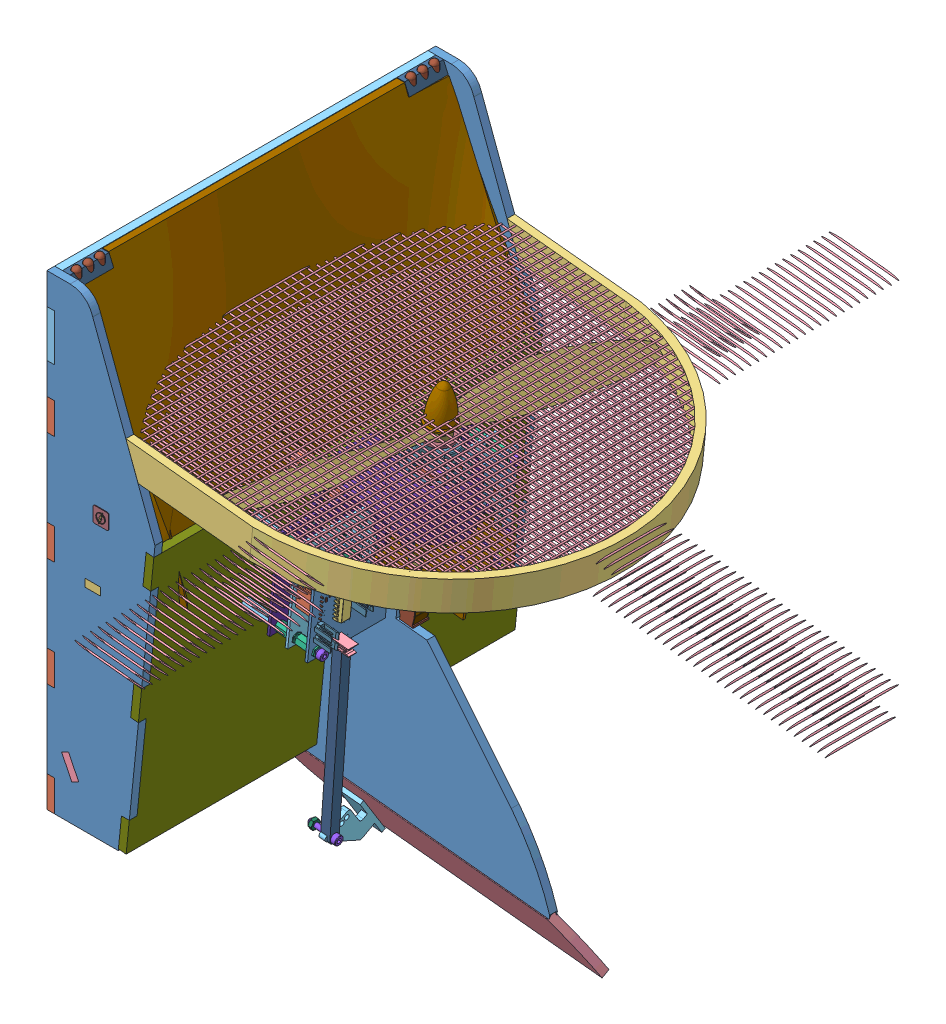
SolidWorks assembly AssTotaleSimu8, configuration Défaut. Lengths in mm. (continued)
Components (placement in the parent): (continued)
- AssStructSimu-1: AssStructSimu [Défaut] at (-125.7658 -1.8483 624.6548) x (1 0 0) z (0 0 -1) size (253.25 324.59 251.6) (continued)
  - AssCarte-1: AssCarte [Défaut] at (-42.8534 32.2132 302.028) x (-0.101852 0.9948 0) z (0.9948 0.101852 0) size (67.15 130.57 98.45) (continued)
    - carte_onduleur_v4-1: carte_onduleur_v4 [Défaut] at (-25.7639 0.8332 112.9379) size (66.52 130.57 82.34) (continued)
      - CARTE_ALIM-1: CARTE_ALIM [Défaut] at (-6.4 -57.2 0.803) size (60 130 18.35) (continued)
        - Open CASCADE STEP translator 6.8 1.63.1-1: Open CASCADE STEP translator 6.8 1.63.1 [Défaut] at origin size (60 130 18.35) (continued)
          - Body_1_6-1: Body_1_6 [Défaut] at (7 56 -12) size (60 130 18.35) (continued)
            - 109-1: 109 [Défaut] at (25.4933 -41.1272 0.803) x (-1 0 0) z (0 0 1) size (2.34 1.04 0.5) (continued)
              - =_[0_1_1_45]-1: =_[0_1_1_45] [Défaut] at origin size (2.34 1.04 0.5) (continued)
                - 49_3-1: 49_3 [Défaut] at origin size (2.29 1.04 0.43)
                - 50-1: 50 [Défaut] at (0.3048 0 0) x (-1 0 0) z (0 0 1) size (0.51 1.02 0.5)
                - 51-1: 51 [Défaut] at origin size (0.51 1.02 0.5)
            - 111-1: 111 [Défaut] at (22.0269 -41.8272 0.803) x (-1 0 0) z (0 0 1) size (2.34 1.04 0.5)
              - =_[0_1_1_45]-1: =_[0_1_1_45] [Défaut] at origin size (2.34 1.04 0.5)
                - 49_3-1: 49_3 [Défaut] at origin size (2.29 1.04 0.43)
                - 50-1: 50 [Défaut] at (0.3048 0 0) x (-1 0 0) z (0 0 1) size (0.51 1.02 0.5)
                - 51-1: 51 [Défaut] at origin size (0.51 1.02 0.5)
            - 113-1: 113 [Défaut] at (-24.8 -36.7036 0.803) x (0 1 0) z (0 0 1) size (2.34 1.04 0.5)
              - =_[0_1_1_45]-1: =_[0_1_1_45] [Défaut] at origin size (2.34 1.04 0.5)
                - 49_3-1: 49_3 [Défaut] at origin size (2.29 1.04 0.43)
                - 50-1: 50 [Défaut] at (0.3048 0 0) x (-1 0 0) z (0 0 1) size (0.51 1.02 0.5)
                - 51-1: 51 [Défaut] at origin size (0.51 1.02 0.5)
            - 115-1: 115 [Défaut] at (-24.8 -40.3036 0.803) x (0 1 0) z (0 0 1) size (2.34 1.04 0.5)
              - =_[0_1_1_45]-1: =_[0_1_1_45] [Défaut] at origin size (2.34 1.04 0.5)
                - 49_3-1: 49_3 [Défaut] at origin size (2.29 1.04 0.43)
                - 50-1: 50 [Défaut] at (0.3048 0 0) x (-1 0 0) z (0 0 1) size (0.51 1.02 0.5)
                - 51-1: 51 [Défaut] at origin size (0.51 1.02 0.5)
            - 117-1: 117 [Défaut] at (-16 -48.27 0.803) x (0 -1 0) z (0 0 1) size (2.34 1.04 0.5)
              - =_[0_1_1_45]-1: =_[0_1_1_45] [Défaut] at origin size (2.34 1.04 0.5)
                - 49_3-1: 49_3 [Défaut] at origin size (2.29 1.04 0.43)
                - 50-1: 50 [Défaut] at (0.3048 0 0) x (-1 0 0) z (0 0 1) size (0.51 1.02 0.5)
                - 51-1: 51 [Défaut] at origin size (0.51 1.02 0.5)
            - 119-1: 119 [Défaut] at (-22.5189 -47.87 0.803) x (-1 0 0) z (0 0 1) size (2.34 1.04 0.5)
              - =_[0_1_1_45]-1: =_[0_1_1_45] [Défaut] at origin size (2.34 1.04 0.5)
                - 49_3-1: 49_3 [Défaut] at origin size (2.29 1.04 0.43)
                - 50-1: 50 [Défaut] at (0.3048 0 0) x (-1 0 0) z (0 0 1) size (0.51 1.02 0.5)
                - 51-1: 51 [Défaut] at origin size (0.51 1.02 0.5)
            - 121-1: 121 [Défaut] at (22.3933 -38.9272 0.803) size (2.34 1.04 0.5)
              - =_[0_1_1_45]-1: =_[0_1_1_45] [Défaut] at origin size (2.34 1.04 0.5)
                - 49_3-1: 49_3 [Défaut] at origin size (2.29 1.04 0.43)
                - 50-1: 50 [Défaut] at (0.3048 0 0) x (-1 0 0) z (0 0 1) size (0.51 1.02 0.5)
                - 51-1: 51 [Défaut] at origin size (0.51 1.02 0.5)
            - 123-1: 123 [Défaut] at (22.0933 -36.4272 0.803) x (-1 0 0) z (0 0 1) size (2.34 1.04 0.5)
              - =_[0_1_1_45]-1: =_[0_1_1_45] [Défaut] at origin size (2.34 1.04 0.5)
                - 49_3-1: 49_3 [Défaut] at origin size (2.29 1.04 0.43)
                - 50-1: 50 [Défaut] at (0.3048 0 0) x (-1 0 0) z (0 0 1) size (0.51 1.02 0.5)
                - 51-1: 51 [Défaut] at origin size (0.51 1.02 0.5)
            - 125-1: 125 [Défaut] at (22.3933 -32.0272 0.803) x (0 -1 0) z (0 0 1) size (2.34 1.04 0.5)
              - =_[0_1_1_45]-1: =_[0_1_1_45] [Défaut] at origin size (2.34 1.04 0.5)
                - 49_3-1: 49_3 [Défaut] at origin size (2.29 1.04 0.43)
                - 50-1: 50 [Défaut] at (0.3048 0 0) x (-1 0 0) z (0 0 1) size (0.51 1.02 0.5)
                - 51-1: 51 [Défaut] at origin size (0.51 1.02 0.5)
            - 127-1: 127 [Défaut] at (17.9597 -23.1272 0.803) size (2.34 1.04 0.5)
              - =_[0_1_1_16]-1: =_[0_1_1_16] [Défaut] at origin size (2.34 1.04 0.5)
                - 14_2-1: 14_2 [Défaut] at origin size (2.29 1.04 0.43)
                - 15_2-1: 15_2 [Défaut] at (0.3048 0 0) x (-1 0 0) z (0 0 1) size (0.51 1.02 0.5)
                - 16_2-1: 16_2 [Défaut] at origin size (0.51 1.02 0.5)
            - 129-1: 129 [Défaut] at (20.0269 -24.9272 0.803) x (-1 0 0) z (0 0 1) size (2.34 1.04 0.5)
              - =_[0_1_1_16]-1: =_[0_1_1_16] [Défaut] at origin size (2.34 1.04 0.5)
                - 14_2-1: 14_2 [Défaut] at origin size (2.29 1.04 0.43)
                - 15_2-1: 15_2 [Défaut] at (0.3048 0 0) x (-1 0 0) z (0 0 1) size (0.51 1.02 0.5)
                - 16_2-1: 16_2 [Défaut] at origin size (0.51 1.02 0.5)
            - 131-1: 131 [Défaut] at (16.9933 -37.5272 0.803) x (-1 0 0) z (0 0 1) size (2.34 1.04 0.5)
              - =_[0_1_1_45]-1: =_[0_1_1_45] [Défaut] at origin size (2.34 1.04 0.5)
                - 49_3-1: 49_3 [Défaut] at origin size (2.29 1.04 0.43)
                - 50-1: 50 [Défaut] at (0.3048 0 0) x (-1 0 0) z (0 0 1) size (0.51 1.02 0.5)
                - 51-1: 51 [Défaut] at origin size (0.51 1.02 0.5)
            - 136-1: 136 [Défaut] at (3.2957 -29.23 0.803) x (-1 0 0) z (0 0 1) size (4.78 2.79 2.03)
              - =_[0_1_1_110]_2-1: =_[0_1_1_110]_2 [Défaut] at origin size (4.78 2.79 2.03)
                - 132-1: 132 [Défaut] at origin size (4.32 2.79 1.78)
                - 133-1: 133 [Défaut] at (0.4572 0 0) x (-1 0 0) z (0 0 1) size (1.02 1.27 1.32)
                - 134-1: 134 [Défaut] at origin size (1.02 1.27 1.32)
            - 141-1: 141 [Défaut] at (0.2436 -33.3673 0.803) size (3.35 1.3 0.55)
              - =_[0_1_1_115]_2-1: =_[0_1_1_115]_2 [Défaut] at origin size (3.35 1.3 0.55)
                - 137-1: 137 [Défaut] at origin size (3.3 1.3 0.48)
                - 138-1: 138 [Défaut] at (0.5588 0 0) x (-1 0 0) z (0 0 1) size (0.76 1.27 0.55)
                - 139-1: 139 [Défaut] at origin size (0.76 1.27 0.55)
            - 143_2-1: 143_2 [Défaut] at (-0.3 -45.47 0.803) x (0 1 0) z (0 0 1) size (2.34 1.04 0.5)
              - =_[0_1_1_16]-1: =_[0_1_1_16] [Défaut] at origin size (2.34 1.04 0.5)
                - 14_2-1: 14_2 [Défaut] at origin size (2.29 1.04 0.43)
                - 15_2-1: 15_2 [Défaut] at (0.3048 0 0) x (-1 0 0) z (0 0 1) size (0.51 1.02 0.5)
                - 16_2-1: 16_2 [Défaut] at origin size (0.51 1.02 0.5)
            - 145-1: 145 [Défaut] at (6.6 31.13 0.803) x (0 1 0) z (0 0 1) size (3.35 1.3 0.55)
              - =_[0_1_1_25]_2-1: =_[0_1_1_25]_2 [Défaut] at origin size (3.35 1.3 0.55)
                - 24-1: 24 [Défaut] at origin size (3.3 1.3 0.48)
                - 25_2-1: 25_2 [Défaut] at (0.5588 0 0) x (-1 0 0) z (0 0 1) size (0.76 1.27 0.55)
                - 26_2-1: 26_2 [Défaut] at origin size (0.76 1.27 0.55)
            - 148-1: 148 [Défaut] at (-7.5 -56.57 0.803) size (15.24 2.54 7.37)
              - =_[0_1_1_122]_2-1: =_[0_1_1_122]_2 [Défaut] at origin size (15.24 2.54 7.37)
                - 146-1: 146 [Défaut] at (6.3 0 1) x (1 0 0) z (0 -1 0) size (15.24 7.37 2.54)
            - 150-1: 150 [Défaut] at (-26.3 -45.9 0.803) x (0 1 0) z (0 0 1) size (2.34 1.04 0.5)
              - =_[0_1_1_45]-1: =_[0_1_1_45] [Défaut] at origin size (2.34 1.04 0.5)
                - 49_3-1: 49_3 [Défaut] at origin size (2.29 1.04 0.43)
                - 50-1: 50 [Défaut] at (0.3048 0 0) x (-1 0 0) z (0 0 1) size (0.51 1.02 0.5)
                - 51-1: 51 [Défaut] at origin size (0.51 1.02 0.5)
    - AssEntretoise-1: AssEntretoise [Défaut] at (-50.7639 -62.5535 129.2811) x (0 0 -1) z (1 0 0) size (58.24 7.29 7.81)
      - socket head cap screw 4762_din-1: socket head cap screw 4762_din [EN ISO 4762 M3 x 5 - 5N] at (-2.4967 0.5867 0) size (8 5.5 5.5)
      - hexagonal_spacer_MF_M3_H20_HEX5.5_FTD6_MTL6-1: hexagonal_spacer_MF_M3_H20_HEX5.5_FTD6_MTL6 [Défaut] at (48.3433 0.5867 0) x (0 0 1) z (-1 0 0) size (6.36 5.51 26)
      - hex nut style 1 gradeab_din-1: hex nut style 1 gradeab_din [Hexagon Nut ISO 4032 - M3 - W - N] at (53.3433 0.5867 0) x (0 0.943962 0.330053) z (-1 0 0) size (5.5 6.35 2.4)
      - hexagonal_spacer_MF_M3_H12_HEX5.5_FTD6_MTL6-2: hexagonal_spacer_MF_M3_H12_HEX5.5_FTD6_MTL6 [Défaut] at (27.0633 0.5867 0) x (0 0.248308 0.968681) z (-1 0 0) size (6.36 5.51 18)
      - hexagonal_spacer_MF_M3_H12_HEX5.5_FTD6_MTL6-3: hexagonal_spacer_MF_M3_H12_HEX5.5_FTD6_MTL6 [Défaut] at (13.7833 0.5867 0) x (0 0 1) z (-1 0 0) size (6.36 5.51 18)
    - AssEntretoise-2: AssEntretoise [Défaut] at (0.4521 -62.0374 129.2811) x (0 0 -1) z (0.694658 0.71934 0) size (58.24 7.29 7.81)
      - socket head cap screw 4762_din-1: socket head cap screw 4762_din [EN ISO 4762 M3 x 5 - 5N] at (-2.4967 0.5867 0) size (8 5.5 5.5)
      - hexagonal_spacer_MF_M3_H20_HEX5.5_FTD6_MTL6-1: hexagonal_spacer_MF_M3_H20_HEX5.5_FTD6_MTL6 [Défaut] at (48.3433 0.5867 0) x (0 0 1) z (-1 0 0) size (6.36 5.51 26)
      - hex nut style 1 gradeab_din-1: hex nut style 1 gradeab_din [Hexagon Nut ISO 4032 - M3 - W - N] at (53.3433 0.5867 0) x (0 0.943962 0.330053) z (-1 0 0) size (5.5 6.35 2.4)
      - hexagonal_spacer_MF_M3_H12_HEX5.5_FTD6_MTL6-2: hexagonal_spacer_MF_M3_H12_HEX5.5_FTD6_MTL6 [Défaut] at (27.0633 0.5867 0) x (0 0.248308 0.968681) z (-1 0 0) size (6.36 5.51 18)
      - hexagonal_spacer_MF_M3_H12_HEX5.5_FTD6_MTL6-3: hexagonal_spacer_MF_M3_H12_HEX5.5_FTD6_MTL6 [Défaut] at (13.7833 0.5867 0) x (0 0 1) z (-1 0 0) size (6.36 5.51 18)
    - AssEntretoise-3: AssEntretoise [Défaut] at (-51.9799 58.1038 129.2811) x (0 0 -1) z (-0.694658 -0.71934 0) size (58.24 7.29 7.81)
      - socket head cap screw 4762_din-1: socket head cap screw 4762_din [EN ISO 4762 M3 x 5 - 5N] at (-2.4967 0.5867 0) size (8 5.5 5.5)
      - hexagonal_spacer_MF_M3_H20_HEX5.5_FTD6_MTL6-1: hexagonal_spacer_MF_M3_H20_HEX5.5_FTD6_MTL6 [Défaut] at (48.3433 0.5867 0) x (0 0 1) z (-1 0 0) size (6.36 5.51 26)
      - hex nut style 1 gradeab_din-1: hex nut style 1 gradeab_din [Hexagon Nut ISO 4032 - M3 - W - N] at (53.3433 0.5867 0) x (0 0.943962 0.330053) z (-1 0 0) size (5.5 6.35 2.4)
      - hexagonal_spacer_MF_M3_H12_HEX5.5_FTD6_MTL6-2: hexagonal_spacer_MF_M3_H12_HEX5.5_FTD6_MTL6 [Défaut] at (27.0633 0.5867 0) x (0 0.248308 0.968681) z (-1 0 0) size (6.36 5.51 18)
      - hexagonal_spacer_MF_M3_H12_HEX5.5_FTD6_MTL6-3: hexagonal_spacer_MF_M3_H12_HEX5.5_FTD6_MTL6 [Défaut] at (13.7833 0.5867 0) x (0 0 1) z (-1 0 0) size (6.36 5.51 18)
    - AssEntretoise-4: AssEntretoise [Défaut] at (0.2897 58.1744 129.2811) x (0 0 -1) z (-0.999848 0.017452 0) size (58.24 7.29 7.81)
      - socket head cap screw 4762_din-1: socket head cap screw 4762_din [EN ISO 4762 M3 x 5 - 5N] at (-2.4967 0.5867 0) size (8 5.5 5.5)
      - hexagonal_spacer_MF_M3_H20_HEX5.5_FTD6_MTL6-1: hexagonal_spacer_MF_M3_H20_HEX5.5_FTD6_MTL6 [Défaut] at (48.3433 0.5867 0) x (0 0 1) z (-1 0 0) size (6.36 5.51 26)
      - hex nut style 1 gradeab_din-1: hex nut style 1 gradeab_din [Hexagon Nut ISO 4032 - M3 - W - N] at (53.3433 0.5867 0) x (0 0.943962 0.330053) z (-1 0 0) size (5.5 6.35 2.4)
      - hexagonal_spacer_MF_M3_H12_HEX5.5_FTD6_MTL6-2: hexagonal_spacer_MF_M3_H12_HEX5.5_FTD6_MTL6 [Défaut] at (27.0633 0.5867 0) x (0 0.248308 0.968681) z (-1 0 0) size (6.36 5.51 18)
      - hexagonal_spacer_MF_M3_H12_HEX5.5_FTD6_MTL6-3: hexagonal_spacer_MF_M3_H12_HEX5.5_FTD6_MTL6 [Défaut] at (13.7833 0.5867 0) x (0 0 1) z (-1 0 0) size (6.36 5.51 18)
    - AssMpu-1: AssMpu [Défaut] at (-44.7921 29.4106 121.7839) size (8 8 22.28)
      - hex nut style 1 gradeab_din-1: hex nut style 1 gradeab_din [Hexagon Nut ISO 4032 - M3 - W - N] at (0.2783 0.3227 1.2) size (5.5 6.35 2.4)
      - plain washer 6903 type ab_din-1: plain washer 6903 type ab_din [DIN 6903-A3] at (0.2783 0.3227 1.2) x (0 0 1) z (-1 0 0) size (1 8 8)
      - socket head cap screw 4762_din-1: socket head cap screw 4762_din [EN ISO 4762 M3 x 5 - 5N] at (0.2783 0.3227 19.76) x (0 0 -1) z (-0.852155 0.523289 0) size (8 5.5 5.5)
      - hexagonal_spacer_MF_M3_H12_HEX5.5_FTD6_MTL6-1: hexagonal_spacer_MF_M3_H12_HEX5.5_FTD6_MTL6 [Défaut] at (0.2783 0.3227 3.48) size (6.36 5.51 18)
    - AssMpu-2: AssMpu [Défaut] at (-24.7921 29.4106 121.7839) size (8 8 22.28)
      - hex nut style 1 gradeab_din-1: hex nut style 1 gradeab_din [Hexagon Nut ISO 4032 - M3 - W - N] at (0.2783 0.3227 1.2) size (5.5 6.35 2.4)
      - plain washer 6903 type ab_din-1: plain washer 6903 type ab_din [DIN 6903-A3] at (0.2783 0.3227 1.2) x (0 0 1) z (-1 0 0) size (1 8 8)
      - socket head cap screw 4762_din-1: socket head cap screw 4762_din [EN ISO 4762 M3 x 5 - 5N] at (0.2783 0.3227 19.76) x (0 0 -1) z (-0.852155 0.523289 0) size (8 5.5 5.5)
      - hexagonal_spacer_MF_M3_H12_HEX5.5_FTD6_MTL6-1: hexagonal_spacer_MF_M3_H12_HEX5.5_FTD6_MTL6 [Défaut] at (0.2783 0.3227 3.48) size (6.36 5.51 18)
    - AssCosse-1: AssCosse [Défaut] at (-36.6204 16.2367 163.5671) x (0 1 0) z (-0.344896 0 0.938641) size (9.83 18.66 11.64)
      - socket head cap screw 4762_din-1: socket head cap screw 4762_din [EN ISO 4762 M3 x 6 - 6N] at (-5.1064 0.3659 0) size (9 5.5 5.5)
      - plain washer 6903 type ab_din-1: plain washer 6903 type ab_din [DIN 6903-A3] at (-2.1064 0.3659 0) size (1 8 8)
      - hex nut style 1 gradeab_din-2: hex nut style 1 gradeab_din [Hexagon Nut ISO 4032 - M3 - W - N] at (1.281 0.3659 0) x (0 0.924225 0.381849) z (-1 0 0) size (5.5 6.35 2.4)
      - 31880-1: 31880 [Default] at (0.4936 0.3659 0) x (0 0.344896 -0.938641) z (0 -0.938641 -0.344896) size (5.54 5 17.37)
    - AssCosse-2: AssCosse [Défaut] at (-36.6204 1.2367 163.5671) x (0 1 0) z (-0.344896 0 0.938641) size (9.83 18.66 11.64)
      - socket head cap screw 4762_din-1: socket head cap screw 4762_din [EN ISO 4762 M3 x 6 - 6N] at (-5.1064 0.3659 0) size (9 5.5 5.5)
      - plain washer 6903 type ab_din-1: plain washer 6903 type ab_din [DIN 6903-A3] at (-2.1064 0.3659 0) size (1 8 8)
      - hex nut style 1 gradeab_din-2: hex nut style 1 gradeab_din [Hexagon Nut ISO 4032 - M3 - W - N] at (1.281 0.3659 0) x (0 0.924225 0.381849) z (-1 0 0) size (5.5 6.35 2.4)
      - 31880-1: 31880 [Default] at (0.4936 0.3659 0) x (0 0.344896 -0.938641) z (0 -0.938641 -0.344896) size (5.54 5 17.37)
    - AssCosse-3: AssCosse [Défaut] at (-36.6204 -13.7633 163.5671) x (0 1 0) z (-0.344896 0 0.938641) size (9.83 18.66 11.64)
      - socket head cap screw 4762_din-1: socket head cap screw 4762_din [EN ISO 4762 M3 x 6 - 6N] at (-5.1064 0.3659 0) size (9 5.5 5.5)
      - plain washer 6903 type ab_din-1: plain washer 6903 type ab_din [DIN 6903-A3] at (-2.1064 0.3659 0) size (1 8 8)
      - hex nut style 1 gradeab_din-2: hex nut style 1 gradeab_din [Hexagon Nut ISO 4032 - M3 - W - N] at (1.281 0.3659 0) x (0 0.924225 0.381849) z (-1 0 0) size (5.5 6.35 2.4)
      - 31880-1: 31880 [Default] at (0.4936 0.3659 0) x (0 0.344896 -0.938641) z (0 -0.938641 -0.344896) size (5.54 5 17.37)
    - Terminal_QD_Female-1: Terminal_QD_Female [Default] at (-33.4139 20.2862 128.1409) x (0 1 0) z (-1 0 0) size (9.4 5.5 22.35)
    - Terminal_QD_Female-2: Terminal_QD_Female [Default] at (-33.4139 5.2862 128.1409) x (0 1 0) z (-1 0 0) size (9.4 5.5 22.35)
    - Terminal_QD_Female-3: Terminal_QD_Female [Default] at (-33.4139 -9.7138 128.1409) x (0 1 0) z (-1 0 0) size (9.4 5.5 22.35)
    - Terminal_QD_Female-4: Terminal_QD_Female [Default] at (-33.4139 -9.7138 145.1409) x (0 1 0) z (-1 0 0) size (9.4 5.5 22.35)
    - Terminal_QD_Female-5: Terminal_QD_Female [Default] at (-33.4139 5.2862 145.1409) x (0 1 0) z (-1 0 0) size (9.4 5.5 22.35)
    - Terminal_QD_Female-6: Terminal_QD_Female [Default] at (-33.4139 20.2862 145.1409) x (0 1 0) z (-1 0 0) size (9.4 5.5 22.35)
- AssTige-1: AssTige [Défaut] at (-241.576 -121.7726 340.4233) x (-0.101791 -0.994204 -0.034587) z (0.9948 -0.101852 0) size (166.39 7.19 19)
  - tige_servo-1: tige_servo [Défaut] at (-106.2712 0.2685 162) size (165 6 6)
  - socket head cap screw 4762_din-2: socket head cap screw 4762_din [EN ISO 4762 M2 x 10 - 10N] at (-104.2712 3.2685 170) x (0 0 -1) z (0.923728 0.383049 0) size (12 3.8 3.8)
  - hex nut style 1 gradeab_din-1: hex nut style 1 gradeab_din [Hexagon Nut ISO 4032 - M3 - W - N] at (55.7288 3.2685 156) size (5.5 6.35 2.4)
  - hex nut style 1 gradeab_din-2: hex nut style 1 gradeab_din [Hexagon Nut ISO 4032 - M2 - W - N] at (-104.2712 3.2685 160) x (0.904801 0.425836 0) z (0 0 1) size (4 4.62 1.6)
  - socket head cap screw 4762_din-3: socket head cap screw 4762_din [EN ISO 4762 M3 x 16 - 16N] at (55.7288 3.2685 171) x (0 0 -1) z (0.923728 0.383049 0) size (19 5.5 5.5)
- AssGoPro-1: AssGoPro [Défaut] at (-119.9926 15.1708 318.2917) x (0 0 -1) z (-0.119031 -0.99289 0) size (64.3 52.3 34.42)
  - GoPRo Frame for LCD Screen-1: GoPRo Frame for LCD Screen [Défaut] at (-2.6935 10.9558 5.5635) size (64.3 47.42 34.42)
    - GoProFrame MJM-1: GoProFrame MJM [Défaut] at (-3.6084 -1.6692 52.45) size (64.3 59.3 23.5)
    - GoPro Hero 3 Front Panel-1: GoPro Hero 3 Front Panel [Défaut] at (-3.6084 -1.6692 55.7) x (-1 0 0) z (0 0 -1) size (59.25 41.2 1.9)
    - GoPro Hero 3 Screen-1: GoPro Hero 3 Screen [Défaut] at (12.7166 3.9308 54.9) size (15 18 1)
    - GoPro Hero 3 Mode Button-1: GoPro Hero 3 Mode Button [Défaut] at (13.4166 -12.4692 54.95) x (-1 0 0) z (0 0 -1) size (11.97 12.11 3.03)
    - GoPro Hero 3 LED Cover-1: GoPro Hero 3 LED Cover [Défaut] at (3.1166 -9.3192 54.85) x (-0.999988 0.004848 0) z (0 0 -1) size (5 5 1.4)
    - GoPro Hero 3 LED Cover-2: GoPro Hero 3 LED Cover [Défaut] at (3.1166 -16.0692 54.85) x (-0.999988 0.004848 0) z (0 0 -1) size (5 5 1.4)
    - GoPro Hero 3 Housing-1: GoPro Hero 3 Housing [Défaut] at (-3.6084 -1.6692 55.7) size (59.37 41.3 29.84)
    - GoPro Hero 3 Lens-1: GoPro Hero 3 Lens [Défaut] at (-18.9334 5.6308 47.35) x (-0.380542 -0.924764 0) z (0 0 -1) size (13.71 15.7 7.94)
    - GoPro Hero 3 Indicator Cover-1: GoPro Hero 3 Indicator Cover [Défaut] at (-25.5834 -22.2692 69.9) x (-0.997412 0 -0.0719) z (0 1 0) size (3 3 2)
    - GoPro Hero 3 Indicator Cover-2: GoPro Hero 3 Indicator Cover [Défaut] at (-28.8834 12.2308 73) x (-0.999992 0.004018 0) z (0 0 1) size (3 3 2)
    - GoPro Hero 3 Indicator Cover-3: GoPro Hero 3 Indicator Cover [Défaut] at (20.6666 16.9308 58.4) x (-0.997739 0 -0.067212) z (0 1 0) size (3 3 2)
    - slot-1: slot [Défaut] at (-24.7434 -9.7363 65.05) x (0 1 0) z (0 0 -1) size (16 15.02 2.44)
    - GoPro Hero 3 HDMI pin-1: GoPro Hero 3 HDMI pin [Défaut] at (-26.982 2.9815 24.7172) x (0.105491 0.98175 -0.158237) z (-0.992872 0.095109 -0.071829) size (3.29 0.86 3.28)
  - support1-2: support1 [Défaut] at (-1.3019 -18.8633 67.0135) x (0 0 1) z (-1 0 0) size (5 5 10)
- AssGouv-1: AssGouv [Défaut] at (-43.2668 -298.2106 479.8345) x (0.9948 -0.101852 0) z (0.055947 0.546439 -0.835628) size (200.18 52.5 43.47)
  - P10_1-1: P10_1 [Défaut] at (-108.1667 -19.4144 197.6829) size (200.18 50.13 5)
  - attache_pale-1: attache_pale [Défaut] at (-49.1667 8.0856 190.1829) x (0 0 -1) z (-1 0 0) size (43.47 35 14)
- Parallax-Servo-Horn-1: Parallax-Servo-Horn [Défaut] at (-69.3162 -29.8353 324.5606) x (0.09792 0.956393 0.27518) z (0.9948 -0.101852 0) size (38.81 38.81 6.17)
- NTM_35-36_engine_assembly-1: NTM_35-36_engine_assembly [Défaut] at (-24.3523 26.8781 325.7101) x (0.9948 -0.101852 0) z (0 0 1) size (60.56 77.2 246.41)
  - engine_base-1: engine_base [Défaut] at (-1.8719 -19.5526 -1.1165) x (0 1 0) z (0 0 1) size (6.8 35 35)
  - engine_bearing-1: engine_bearing [Défaut] at origin size (10 4 10)
  - Propeller_cone-1: Propeller_cone [Défaut] at (-1.8719 33.6474 -4.1165) x (1 0 0) z (0 1 0) size (17.6 17.6 24)
  - engine_bearing-2: engine_bearing [Défaut] at (0 22.8 0) size (10 4 10)
  - NTM_35-36_enginebody-1: NTM_35-36_enginebody [Défaut] at (-1.8719 -12.7526 -1.1165) size (35 31.7 35)
  - Stator-1: Stator [Défaut] at origin size (27.75 22.36 27.94)
  - propellers_10x4-1: propellers_10x4 [Défaut] at (-6.8719 27.4474 -4.9165) size (60.56 10.53 246.41)
  - propeller_washer-1: propeller_washer [Défaut] at (-1.8719 24.4474 -1.1165) x (0 1 0) z (0 0 1) size (2.5 18 18)
  - Propeller_adaptor-1: Propeller_adaptor [Défaut] at (2.1948 17.1101 -3.713) size (23.46 32.5 25)
Mates (geometry in assembly coordinates):
- Coaxiale1: concentric aligned: cylinder of AssStructSimu-1/AssToitMot-1/AssToit-1/P12-1 through (-27.6967 12.5918 324.5936) axis (-0.101852 -0.9948 0) radius 17.5; cylinder of NTM_35-36_engine_assembly-1/NTM_35-36_enginebody-1 through (-25.2217 36.7654 324.5936) axis (-0.101852 -0.9948 0) radius 17.5
- Coïncidente1: coincident anti-aligned: plane of AssStructSimu-1/AssToitMot-1/AssToit-1/P12-1 through (-28.206 7.6178 324.5936) normal (0.101852 0.9948 0); plane of NTM_35-36_engine_assembly-1/engine_bearing-1 through (-28.206 7.6178 324.5936) normal (-0.101852 -0.9948 0)
- Coaxiale2: concentric aligned: cylinder of AssStructSimu-1/AssToitMot-1/AssToit-1/P10_2-1 through (49.7135 -178.7878 324.5936) axis (-0.9948 0.101852 0) radius 2.5; cylinder of AssGouv-1/P10_1-1 through (-94.0351 -164.0702 324.5936) axis (-0.9948 0.101852 0) radius 2.5
- Coïncidente2: coincident aligned: plane of AssStructSimu-1/AssToitMot-1/AssToit-1/P10_2-1 through (-137.5516 -157.1017 322.0936) normal (-0.9948 0.101852 0); plane of AssGouv-1/P10_1-1 through (-137.8791 -160.3008 321.1312) normal (-0.9948 0.101852 0)
- Coaxiale3: concentric aligned: cylinder of AssTige-1/socket head cap screw 4762_din-3 through (-45.5416 -197.7164 335.2292) axis (0.9948 -0.101852 0) radius 1.5; cylinder of AssGouv-1/attache_pale-1 through (-85.9983 -193.5742 335.2292) axis (0.9948 -0.101852 0) radius 1.5
- Coaxiale4: concentric aligned: cylinder of AssStructSimu-1/AssToitMot-1/Parallax-Servo_DUMMY-1 through (-70.6554 -29.6982 324.5606) axis (-0.9948 0.101852 0) radius 2.9845; cylinder of Parallax-Servo-Horn-1 through (-70.6554 -29.6982 324.5606) axis (-0.9948 0.101852 0) radius 2.9845
- Coïncidente3: coincident anti-aligned: plane of AssStructSimu-1/AssToitMot-1/Parallax-Servo_DUMMY-1 through (-74.8246 -29.2713 324.5606) normal (0.9948 -0.101852 0); plane of Parallax-Servo-Horn-1 through (-74.8246 -29.2713 324.5606) normal (-0.9948 0.101852 0)
- Coaxiale5: concentric anti-aligned: cylinder of AssTige-1/socket head cap screw 4762_din-2 through (-30.2498 -38.5418 340.7631) axis (0.9948 -0.101852 0) radius 1; cylinder of Parallax-Servo-Horn-1 through (-69.7931 -34.4932 340.7631) axis (-0.9948 0.101852 0) radius 0.635
- Coïncidente4: coincident anti-aligned: plane of AssTige-1/tige_servo-1 through (-69.6001 -32.608 343.8305) normal (-0.9948 0.101852 0); plane of Parallax-Servo-Horn-1 through (-68.8748 -25.5237 332.3708) normal (0.9948 -0.101852 0)
- Coaxiale6: concentric aligned: cylinder of AssStructSimu-1/AssBase-1/socket head cap screw 4762_din-7 through (-144.5139 -51.9008 369.3436) axis (0 0 1) radius 1.5; cylinder of AssGoPro-1/support1-2 through (-144.5139 -51.9008 319.5936) axis (0 0 1) radius 1.5
- Coïncidente5: coincident anti-aligned: plane of AssStructSimu-1/AssBase-1/support2-1 through (-141.9706 -54.3568 329.5936) normal (0 0 -1); plane of AssGoPro-1/support1-2 through (-146.6985 -49.121 329.5936) normal (0 0 1)
